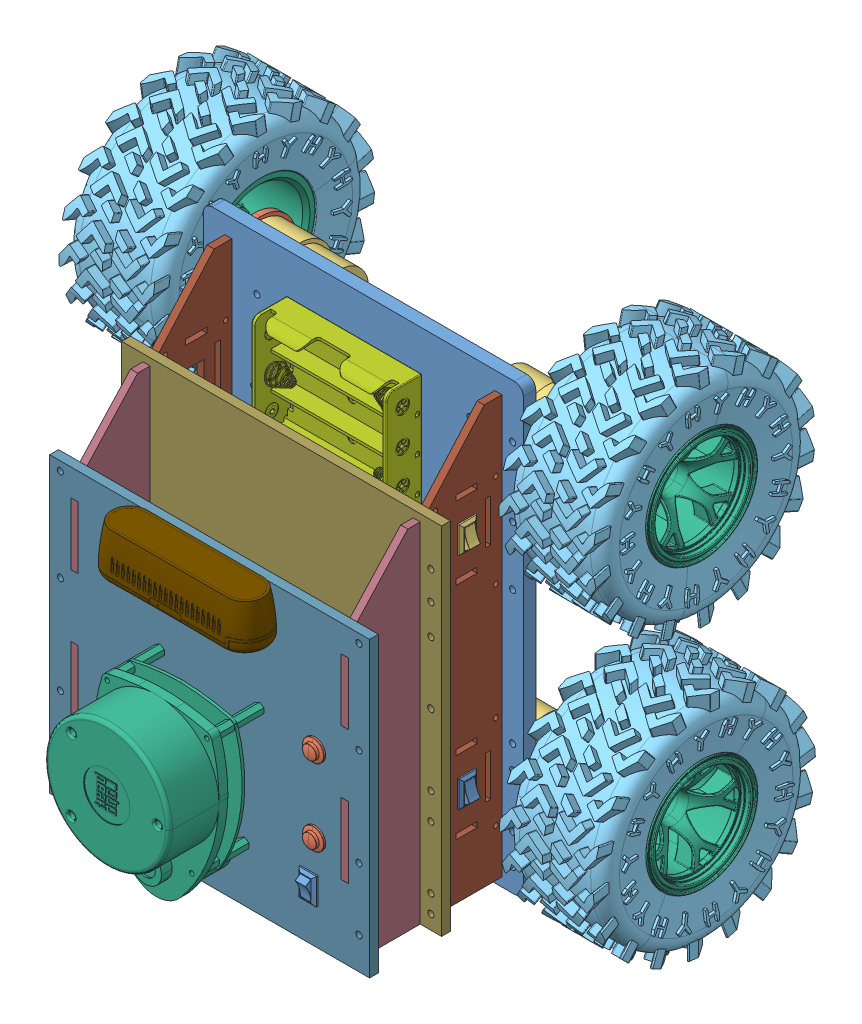
SolidWorks assembly Assem1, configuration Default. Lengths in mm. (continued)
Mates (geometry in assembly coordinates): (continued)
- Coincident108: coincident anti-aligned: plane of BTS_driver-4 through (-152.8182 1209.5505 -471.1522) normal (0 0 1); plane of Copy of hexagonal_spacer_FF_M3_H05_HEX5_pass_through.step^Assem1-4 through (-175.8052 1191.8975 -471.1522) normal (0 0 -1)
- Concentric77: concentric anti-aligned: cylinder of BTS_driver-4 through (-175.8052 1227.4575 -470.3622) axis (0 0 -1) radius 1.75; cylinder of Copy of hexagonal_spacer_FF_M3_H05_HEX5_pass_through.step^Assem1-5 through (-175.8052 1227.4575 -470.8751) axis (0 0 1) radius 1.5
- Coincident109: coincident anti-aligned: plane of BTS_driver-4 through (-152.8182 1209.5505 -471.1522) normal (0 0 1); plane of Copy of hexagonal_spacer_FF_M3_H05_HEX5_pass_through.step^Assem1-5 through (-175.8052 1227.4575 -471.1522) normal (0 0 -1)
- Concentric78: concentric anti-aligned: cylinder of BTS_driver-4 through (-130.0852 1227.4575 -470.3622) axis (0 0 -1) radius 1.75; cylinder of Copy of hexagonal_spacer_FF_M3_H05_HEX5_pass_through.step^Assem1-6 through (-130.0852 1227.4575 -470.8751) axis (0 0 1) radius 1.5
- Coincident110: coincident anti-aligned: plane of BTS_driver-4 through (-152.8182 1209.5505 -471.1522) normal (0 0 1); plane of Copy of hexagonal_spacer_FF_M3_H05_HEX5_pass_through.step^Assem1-6 through (-130.0852 1227.4575 -471.1522) normal (0 0 -1)
- Concentric79: concentric anti-aligned: cylinder of BTS_driver-4 through (-130.0852 1191.8975 -470.3622) axis (0 0 -1) radius 1.75; cylinder of Copy of hexagonal_spacer_FF_M3_H05_HEX5_pass_through.step^Assem1-7 through (-130.0852 1191.8975 -470.8751) axis (0 0 1) radius 1.5
- Coincident111: coincident anti-aligned: plane of BTS_driver-4 through (-152.8182 1209.5505 -471.1522) normal (0 0 1); plane of Copy of hexagonal_spacer_FF_M3_H05_HEX5_pass_through.step^Assem1-7 through (-130.0852 1191.8975 -471.1522) normal (0 0 -1)
- Concentric80: concentric anti-aligned: cylinder of BTS_driver-2 through (-253.5052 1290.2975 -470.3622) axis (0 0 -1) radius 1.75; cylinder of Copy of hexagonal_spacer_FF_M3_H05_HEX5_pass_through.step^Assem1-13 through (-253.5052 1290.2975 -470.8751) axis (0 0 1) radius 1.5
- Coincident112: coincident anti-aligned: plane of BTS_driver-2 through (-230.7722 1272.6445 -471.1522) normal (0 0 1); plane of Copy of hexagonal_spacer_FF_M3_H05_HEX5_pass_through.step^Assem1-13 through (-253.5052 1290.2975 -471.1522) normal (0 0 -1)
- Coincident113: coincident anti-aligned: plane of BTS_driver-2 through (-230.7722 1272.6445 -471.1522) normal (0 0 1); plane of Copy of hexagonal_spacer_FF_M3_H05_HEX5_pass_through.step^Assem1-12 through (-207.7852 1290.2975 -471.1522) normal (0 0 -1)
- Concentric81: concentric anti-aligned: cylinder of BTS_driver-2 through (-207.7852 1290.2975 -470.3622) axis (0 0 -1) radius 1.75; cylinder of Copy of hexagonal_spacer_FF_M3_H05_HEX5_pass_through.step^Assem1-12 through (-207.7852 1290.2975 -470.8751) axis (0 0 1) radius 1.5
- Concentric82: concentric anti-aligned: cylinder of BTS_driver-2 through (-207.7852 1254.7375 -470.3622) axis (0 0 -1) radius 1.75; cylinder of Copy of hexagonal_spacer_FF_M3_H05_HEX5_pass_through.step^Assem1-11 through (-207.7852 1254.7375 -470.8751) axis (0 0 1) radius 1.5
- Coincident114: coincident anti-aligned: plane of BTS_driver-2 through (-230.7722 1272.6445 -471.1522) normal (0 0 1); plane of Copy of hexagonal_spacer_FF_M3_H05_HEX5_pass_through.step^Assem1-11 through (-207.7852 1254.7375 -471.1522) normal (0 0 -1)
- Concentric83: concentric anti-aligned: cylinder of BTS_driver-2 through (-253.5052 1254.7375 -470.3622) axis (0 0 -1) radius 1.75; cylinder of Copy of hexagonal_spacer_FF_M3_H05_HEX5_pass_through.step^Assem1-10 through (-253.5052 1254.7375 -470.8751) axis (0 0 1) radius 1.5
- Coincident115: coincident anti-aligned: plane of BTS_driver-2 through (-230.7722 1272.6445 -471.1522) normal (0 0 1); plane of Copy of hexagonal_spacer_FF_M3_H05_HEX5_pass_through.step^Assem1-10 through (-253.5052 1254.7375 -471.1522) normal (0 0 -1)
- Concentric84: concentric anti-aligned: cylinder of BTS_driver-5 through (-207.7852 1227.4575 -470.3622) axis (0 0 -1) radius 1.75; cylinder of Copy of hexagonal_spacer_FF_M3_H05_HEX5_pass_through.step^Assem1-14 through (-207.7852 1227.4575 -470.8751) axis (0 0 1) radius 1.5
- Concentric86: concentric anti-aligned: cylinder of BTS_driver-5 through (-253.5052 1191.8975 -470.3622) axis (0 0 -1) radius 1.75; cylinder of Copy of hexagonal_spacer_FF_M3_H05_HEX5_pass_through.step^Assem1-15 through (-253.5052 1191.8975 -470.8751) axis (0 0 1) radius 1.5
- Concentric87: concentric aligned: cylinder of BTS_driver-5 through (-207.7852 1191.8975 -470.3622) axis (0 0 -1) radius 1.75; circle of Copy of hexagonal_spacer_FF_M3_H05_HEX5_pass_through.step^Assem1-9
- Coincident116: coincident anti-aligned: plane of BTS_driver-5 through (-230.7722 1209.8045 -471.1522) normal (0 0 1); plane of Copy of hexagonal_spacer_FF_M3_H05_HEX5_pass_through.step^Assem1-14 through (-207.7852 1227.4575 -471.1522) normal (0 0 -1)
- Coincident117: coincident anti-aligned: plane of BTS_driver-5 through (-230.7722 1209.8045 -471.1522) normal (0 0 1); plane of Copy of hexagonal_spacer_FF_M3_H05_HEX5_pass_through.step^Assem1-9 through (-207.7852 1191.8975 -471.1522) normal (0 0 -1)
- Coincident118: coincident anti-aligned: plane of BTS_driver-5 through (-230.7722 1209.8045 -471.1522) normal (0 0 1); plane of Copy of hexagonal_spacer_FF_M3_H05_HEX5_pass_through.step^Assem1-15 through (-253.5052 1191.8975 -471.1522) normal (0 0 -1)
- Coincident120: coincident anti-aligned: plane of Tam_lot_motorLon-2 through (-191.7952 1241.0975 -466.1522) normal (0 0 -1); plane of Copy of hexagonal_spacer_FF_M3_H05_HEX5_pass_through.step^Assem1-6 through (-130.0852 1227.4575 -466.1522) normal (0 0 1)
- Coincident121: coincident anti-aligned: plane of Tam_lot_motorLon-2 through (-191.7952 1241.0975 -466.1522) normal (0 0 -1); plane of Copy of hexagonal_spacer_FF_M3_H05_HEX5_pass_through.step^Assem1-2 through (-130.0852 1254.7375 -466.1522) normal (0 0 1)
- Coincident122: coincident anti-aligned: plane of Tam_lot_motorLon-2 through (-191.7952 1241.0975 -466.1522) normal (0 0 -1); plane of Copy of hexagonal_spacer_FF_M3_H05_HEX5_pass_through.step^Assem1-14 through (-207.7852 1227.4575 -466.1522) normal (0 0 1)
- Concentric88: concentric anti-aligned: cylinder of BTS_driver-5 through (-253.5052 1227.4575 -470.3622) axis (0 0 -1) radius 1.75; cylinder of Copy of hexagonal_spacer_FF_M3_H05_HEX5_pass_through.step^Assem1-16 through (-253.5052 1227.4575 -470.8751) axis (0 0 1) radius 1.5
- Coincident124: coincident anti-aligned: plane of BTS_driver-5 through (-230.7722 1209.8045 -471.1522) normal (0 0 1); plane of Copy of hexagonal_spacer_FF_M3_H05_HEX5_pass_through.step^Assem1-16 through (-253.5052 1227.4575 -471.1522) normal (0 0 -1)
- Coincident125: coincident anti-aligned: plane of Tam_lot_motorLon-2 through (-191.7952 1241.0975 -466.1522) normal (0 0 -1); plane of Copy of hexagonal_spacer_FF_M3_H05_HEX5_pass_through.step^Assem1-10 through (-253.5052 1254.7375 -466.1522) normal (0 0 1)
- Parallel37: parallel anti-aligned: line of BTS_driver-2 through (-256.2992 1252.1975 -472.7322) axis (1 0 0); line of BTS_driver-5 through (-205.2452 1230.2515 -472.7322) axis (-1 0 0)
- Parallel38: parallel anti-aligned: line of BTS_driver-2 through (-205.2452 1252.1975 -472.7322) axis (0 1 0); line of BTS_driver-3 through (-178.3452 1292.8375 -472.7322) axis (0 -1 0)
- Parallel39: parallel anti-aligned: line of BTS_driver-4 through (-178.3452 1229.9975 -472.7322) axis (0 -1 0); line of BTS_driver-5 through (-205.2452 1189.3575 -472.7322) axis (0 1 0)
- Parallel40: parallel aligned: line of Tam_lot_motorLon-2 through (-281.7952 1361.0975 -466.1522) axis (0 -1 0); line of BTS_driver-2 through (-256.2992 1293.0915 -472.7322) axis (0 -1 0)
- Concentric91: concentric anti-aligned: cylinder of Tam_lot_motorLon-2 through (-253.5052 1227.4575 -454.2591) axis (0 0 -1) radius 1.73; cylinder of Copy of hexagonal_spacer_FF_M3_H05_HEX5_pass_through.step^Assem1-16 through (-253.5052 1227.4575 -470.8751) axis (0 0 1) radius 1.5
- Concentric92: concentric anti-aligned: cylinder of Tam_lot_motorLon-2 through (-253.5052 1290.2975 -454.2591) axis (0 0 -1) radius 1.73; cylinder of Copy of hexagonal_spacer_FF_M3_H05_HEX5_pass_through.step^Assem1-13 through (-253.5052 1290.2975 -470.8751) axis (0 0 1) radius 1.5
- Concentric93: concentric anti-aligned: cylinder of Tam_lot_motorLon-2 through (-175.8052 1227.4575 -454.2591) axis (0 0 -1) radius 1.73; cylinder of Copy of hexagonal_spacer_FF_M3_H05_HEX5_pass_through.step^Assem1-5 through (-175.8052 1227.4575 -470.8751) axis (0 0 1) radius 1.5
- Concentric94: concentric anti-aligned: cylinder of Tam_lot_motorLon-2 through (-175.8052 1254.7375 -454.2591) axis (0 0 -1) radius 1.73; cylinder of Copy of hexagonal_spacer_FF_M3_H05_HEX5_pass_through.step^Assem1-1 through (-175.8052 1254.7375 -470.8751) axis (0 0 1) radius 1.5
- Concentric95: concentric anti-aligned: cylinder of LM2596-4 through (-151.9594 1232.9725 -452.4522) axis (0 0 -1) radius 1.475; cylinder of Copy of hexagonal_spacer_FF_M3_H05_HEX5_pass_through.step^Assem1-22 through (-151.9594 1232.9725 -458.8751) axis (0 0 1) radius 1.5
- Coincident133: coincident anti-aligned: plane of LM2596-4 through (-167.0594 1241.0975 -454.1522) normal (0 0 -1); plane of Copy of hexagonal_spacer_FF_M3_H05_HEX5_pass_through.step^Assem1-22 through (-151.9594 1232.9725 -454.1522) normal (0 0 1)
- Concentric96: concentric anti-aligned: cylinder of Copy of hexagonal_spacer_FF_M3_H05_HEX5_pass_through.step^Assem1-17 through (-182.1594 1249.2225 -458.8751) axis (0 0 1) radius 1.5; cylinder of LM2596-4 through (-182.1594 1249.2225 -452.4522) axis (0 0 -1) radius 1.475
- Coincident134: coincident anti-aligned: plane of Copy of hexagonal_spacer_FF_M3_H05_HEX5_pass_through.step^Assem1-17 through (-182.1594 1249.2225 -454.1522) normal (0 0 1); plane of LM2596-4 through (-167.0594 1241.0975 -454.1522) normal (0 0 -1)
- Concentric98: concentric anti-aligned: cylinder of Copy of hexagonal_spacer_FF_M3_H05_HEX5_pass_through.step^Assem1-18 through (-202.0152 1232.9725 -458.8751) axis (0 0 1) radius 1.5; cylinder of LM2596-3 through (-202.0152 1232.9725 -452.4522) axis (0 0 -1) radius 1.475
- Coincident135: coincident anti-aligned: plane of Copy of hexagonal_spacer_FF_M3_H05_HEX5_pass_through.step^Assem1-18 through (-202.0152 1232.9725 -454.1522) normal (0 0 1); plane of LM2596-3 through (-217.1152 1241.0975 -454.1522) normal (0 0 -1)
- Coincident136: coincident anti-aligned: plane of Copy of hexagonal_spacer_FF_M3_H05_HEX5_pass_through.step^Assem1-21 through (-232.2152 1249.2225 -454.1522) normal (0 0 1); plane of LM2596-3 through (-217.1152 1241.0975 -454.1522) normal (0 0 -1)
- Concentric99: concentric anti-aligned: cylinder of Copy of hexagonal_spacer_FF_M3_H05_HEX5_pass_through.step^Assem1-21 through (-232.2152 1249.2225 -458.8751) axis (0 0 1) radius 1.5; cylinder of LM2596-3 through (-232.2152 1249.2225 -452.4522) axis (0 0 -1) radius 1.475
- Coincident137: coincident anti-aligned: plane of Tam_lot_motorLon-2 through (-191.7952 1241.0975 -459.1522) normal (0 0 1); plane of Copy of hexagonal_spacer_FF_M3_H05_HEX5_pass_through.step^Assem1-21 through (-232.2152 1249.2225 -459.1522) normal (0 0 -1)
- Coincident138: coincident anti-aligned: plane of Tam_lot_motorLon-2 through (-191.7952 1241.0975 -459.1522) normal (0 0 1); plane of Copy of hexagonal_spacer_FF_M3_H05_HEX5_pass_through.step^Assem1-22 through (-151.9594 1232.9725 -459.1522) normal (0 0 -1)
- Parallel41: parallel aligned: plane of Tam_lot_motorLon-2 through (-281.7952 1116.0975 -459.1522) normal (0 -1 0); plane of Copy of 18650 Cell Holder^Assem1-1 through (-231.0952 1140.7125 -454.1522) normal (0 -1 0)
- Parallel42: parallel aligned: plane of Tam_lot_motorLon-2 through (-281.7952 1116.0975 -459.1522) normal (0 -1 0); plane of Copy of 18650 Cell Holder^Assem1-1 through (-231.0952 1140.7125 -454.1522) normal (0 -1 0)
- Parallel43: parallel aligned: plane of Tam_lot_motorLon-2 through (-281.7952 1366.0975 -459.1522) normal (0 1 0); plane of khay_pin-4/Assem_done(2)^khay_pin-1/18650 Cell Holder^Assem_done(2)_khay_pin-1 through (-152.4952 1341.4825 -459.1522) normal (0 1 0)
- Concentric106: concentric aligned: cylinder of Tam_lot_motorLon-2 through (-202.0152 1232.9725 -454.2591) axis (0 0 -1) radius 1.73; cylinder of LM2596-3 through (-202.0152 1232.9725 -452.4522) axis (0 0 -1) radius 1.475
- Concentric107: concentric aligned: cylinder of Tam_lot_motorLon-2 through (-232.2152 1249.2225 -454.2591) axis (0 0 -1) radius 1.73; cylinder of LM2596-3 through (-232.2152 1249.2225 -452.4522) axis (0 0 -1) radius 1.475
- Concentric108: concentric anti-aligned: cylinder of Tam_lot_motorLon-2 through (-182.1594 1249.2225 -454.2591) axis (0 0 -1) radius 1.73; cylinder of Copy of hexagonal_spacer_FF_M3_H05_HEX5_pass_through.step^Assem1-17 through (-182.1594 1249.2225 -456.6522) axis (0 0 1) radius 1.5
- Concentric109: concentric anti-aligned: cylinder of Tam_lot_motorLon-2 through (-151.9594 1232.9725 -454.2591) axis (0 0 -1) radius 1.73; cylinder of Copy of hexagonal_spacer_FF_M3_H05_HEX5_pass_through.step^Assem1-22 through (-151.9594 1232.9725 -458.8751) axis (0 0 1) radius 1.5
- Parallel45: parallel aligned: plane of Tam_lot_motorLon-2 through (-281.7952 1366.0975 -459.1522) normal (0 1 0); plane of khay_pin-4/Assem_done(2)^khay_pin-1/18650 Cell Holder^Assem_done(2)_khay_pin-1 through (-152.4952 1341.4825 -459.1522) normal (0 1 0)
- Parallel46: parallel aligned: plane of Tam_lot_motorLon-2 through (-101.7952 1366.0975 -459.1522) normal (1 0 0); plane of mat_ben_co_sac-2 through (-113.7952 1238.5975 -459.1522) normal (1 0 0)
- Coincident155: coincident anti-aligned: plane of Tam_lot_motorLon-2 through (-113.7952 1121.0975 -478.8013) normal (0 1 0); plane of mat_ben_co_sac-2 through (-113.7952 1121.0975 -459.1522) normal (0 -1 0)
- Coincident156: coincident anti-aligned: plane of Tam_lot_motorLon-2 through (-113.7952 1133.0975 -478.8013) normal (-1 0 0); plane of mat_ben_co_sac-2 through (-113.7952 1238.5975 -459.1522) normal (1 0 0)
- Coincident157: coincident aligned: plane of Tam_lot_motorLon-2 through (-191.7952 1241.0975 -466.1522) normal (0 0 -1); plane of mat_ben_co_sac-2 through (-113.7952 1133.0975 -466.1522) normal (0 0 -1)
- Coincident158: coincident aligned: plane of Tam_lot_motorLon-2 through (-191.7952 1241.0975 -466.1522) normal (0 0 -1); plane of mat_ben_co_sac-1 through (-265.7952 1133.0975 -466.1522) normal (0 0 -1)
- Parallel47: parallel aligned: plane of Tam_lot_motorLon-2 through (-281.7952 1116.0975 -459.1522) normal (0 -1 0); plane of mat_ben_co_sac-1 through (-265.7952 1121.0975 -459.1522) normal (0 -1 0)
- Coincident160: coincident anti-aligned: plane of Tam_lot_motorLon-2 through (-269.7952 1133.0975 -478.8013) normal (1 0 0); plane of mat_ben_co_sac-1 through (-269.7952 1238.5975 -459.1522) normal (-1 0 0)
- Coincident161: coincident anti-aligned: plane of Tam_lot_motorLon-2 through (-269.7952 1121.0975 -478.8013) normal (0 1 0); plane of mat_ben_co_sac-1 through (-265.7952 1121.0975 -459.1522) normal (0 -1 0)
- Coincident162: coincident anti-aligned: plane of mat_ben_co_sac-1 through (-269.7952 1238.5975 -459.1522) normal (-1 0 0); plane of tang2_2-2 through (-269.7952 1216.0975 -438.5483) normal (1 0 0)
- Coincident163: coincident anti-aligned: plane of mat_ben_co_sac-1 through (-265.7952 1301.0975 -413.1522) normal (0 1 0); plane of tang2_2-2 through (-265.7952 1301.0975 -433.6764) normal (0 -1 0)
- Coincident164: coincident aligned: plane of mat_ben_co_sac-2 through (-113.7952 1146.0975 -413.1522) normal (0 0 1); plane of tang2_2-2 through (-191.7952 1221.0975 -413.1522) normal (0 0 1)
- Coincident166: coincident anti-aligned: plane of tang2_2-2 through (-265.7952 1317.0975 -428.9226) normal (0 -1 0); plane of mat_ben_tang_2-1 through (-265.7952 1317.0975 -413.1522) normal (0 1 0)
- Coincident167: coincident anti-aligned: plane of tang2_2-2 through (-269.7952 1317.0975 -428.9226) normal (1 0 0); plane of mat_ben_tang_2-1 through (-269.7952 1221.0975 -413.1522) normal (-1 0 0)
- Coincident170: coincident aligned: plane of tang2_2-2 through (-191.7952 1221.0975 -418.1522) normal (0 0 -1); plane of mat_ben_tang_2-1 through (-265.7952 1311.0975 -418.1522) normal (0 0 -1)
- Coincident171: coincident anti-aligned: plane of tang2_2-2 through (-117.7952 1317.0975 -428.9226) normal (0 -1 0); plane of mat_ben_tang_2-2 through (-113.7952 1317.0975 -413.1522) normal (0 1 0)
- Coincident172: coincident anti-aligned: plane of tang2_2-2 through (-117.7952 1311.0975 -428.9226) normal (1 0 0); plane of mat_ben_tang_2-2 through (-117.7952 1221.0975 -413.1522) normal (-1 0 0)
- Coincident173: coincident aligned: plane of tang2_2-2 through (-191.7952 1221.0975 -418.1522) normal (0 0 -1); plane of mat_ben_tang_2-2 through (-113.7952 1125.0975 -418.1522) normal (0 0 -1)
- Coincident174: coincident anti-aligned: plane of mat_ben_tang_2-2 through (-113.7952 1271.0975 -372.6522) normal (0 1 0); plane of tang_3-1 through (-117.7952 1271.0975 -412.8801) normal (0 -1 0)
- Coincident175: coincident anti-aligned: plane of mat_ben_tang_2-2 through (-113.7952 1221.0975 -413.1522) normal (1 0 0); plane of tang_3-1 through (-113.7952 1161.0975 -417.8517) normal (-1 0 0)
- Coincident177: coincident aligned: plane of mat_ben_tang_2-2 through (-113.7952 1161.0975 -372.6522) normal (0 0 1); plane of tang_3-1 through (-191.7952 1203.5975 -372.6522) normal (0 0 1)
- Concentric121: concentric anti-aligned: cylinder of tang2_2-2 through (-167.2952 1217.5975 -422.3949) axis (0 0 1) radius 1.5; cylinder of Copy (4) of hexagonal_spacer_FF_M3_H05_HEX5_pass_through.step^Assem1-4 through (-167.2952 1217.5975 -408.4294) axis (0 0 -1) radius 1.5
- Concentric122: concentric anti-aligned: cylinder of tang2_2-2 through (-216.2952 1217.5975 -422.3949) axis (0 0 1) radius 1.5; cylinder of Copy (2) of hexagonal_spacer_FF_M3_H05_HEX5_pass_through.step^Assem1-2 through (-216.2952 1217.5975 -408.4294) axis (0 0 -1) radius 1.5
- Coincident182: coincident anti-aligned: plane of tang2_2-2 through (-191.7952 1221.0975 -413.1522) normal (0 0 1); plane of Copy (4) of hexagonal_spacer_FF_M3_H05_HEX5_pass_through.step^Assem1-4 through (-167.2952 1217.5975 -413.1522) normal (0 0 -1)
- Coincident187: coincident anti-aligned: plane of tang_3-1 through (-191.7952 1203.5975 -372.6522) normal (0 0 1); plane of IntelRealsense_D435_Multibody-1 through (-162.0261 1272.6733 -372.6522) normal (0 0 -1)
- Coincident188: coincident anti-aligned: plane of mat_ben_co_sac-2 through (-134.2257 1167.0975 -434.8522) normal (0 0 -1); plane of swith_on_off-1/Assem_done(2)^swith_on_off-1/Switch on off^Assem_done(2)_swith_on_off-1 through (-111.7952 1180.9706 -434.8522) normal (0 0 1)
- Coincident190: coincident anti-aligned: plane of mat_ben_co_sac-2 through (-113.7952 1238.5975 -459.1522) normal (1 0 0); plane of swith_on_off-1/Assem_done(2)^swith_on_off-1/Switch on off^Assem_done(2)_swith_on_off-1 through (-113.7952 1167.3306 -434.8522) normal (-1 0 0)
- Lock3: lock: unknown of mat_ben_co_sac-2; unknown of swith_on_off-1/Assem_done(2)^swith_on_off-1/Switch on off^Assem_done(2)_swith_on_off-1
- Coincident192: coincident anti-aligned: plane of mat_ben_co_sac-2 through (-134.2257 1291.0975 -434.8522) normal (0 0 -1); plane of Copy of Switch on off^Assem1-1 through (-111.7952 1304.8258 -434.8522) normal (0 0 1)
- Coincident193: coincident anti-aligned: plane of mat_ben_co_sac-2 through (-113.7952 1238.5975 -459.1522) normal (1 0 0); plane of Copy of Switch on off^Assem1-1 through (-113.7952 1291.1858 -434.8522) normal (-1 0 0)
- Lock4: lock: unknown of mat_ben_co_sac-2; unknown of Copy of Switch on off^Assem1-1
- Concentric123: concentric anti-aligned: cylinder of hexagone M3-2/Assem_done(2)^hexagone M3-1/hexagonal_spacer_FF_M3_H05_HEX5_pass_through.step^Assem_done(2)_hexagone M3-3 through (-167.2952 1159.5975 -409.4294) axis (0 0 -1) radius 1.5; cylinder of raspberry pi 4-2/Assem_done(2)^raspberry pi 4-1/Raspberry Pi 4 Model B^Assem_done(2)_raspberry pi 4-1 through (-167.2952 1159.5975 -406.5622) axis (0 0 1) radius 1.35
- Concentric124: concentric anti-aligned: cylinder of Copy (3) of hexagonal_spacer_FF_M3_H05_HEX5_pass_through.step^Assem1-3 through (-216.2952 1159.5975 -409.2374) axis (0 0 -1) radius 1.5; cylinder of raspberry pi 4-2/Assem_done(2)^raspberry pi 4-1/Raspberry Pi 4 Model B^Assem_done(2)_raspberry pi 4-1 through (-216.2952 1159.5975 -406.5622) axis (0 0 1) radius 1.35
- Concentric125: concentric anti-aligned: cylinder of Copy (2) of hexagonal_spacer_FF_M3_H05_HEX5_pass_through.step^Assem1-2 through (-216.2952 1217.5975 -408.4294) axis (0 0 -1) radius 1.5; cylinder of raspberry pi 4-2/Assem_done(2)^raspberry pi 4-1/Raspberry Pi 4 Model B^Assem_done(2)_raspberry pi 4-1 through (-216.2952 1217.5975 -406.5622) axis (0 0 1) radius 1.35
- Concentric126: concentric anti-aligned: cylinder of tang2_2-2 through (-216.2952 1159.5975 -422.3949) axis (0 0 1) radius 1.5; cylinder of Copy (3) of hexagonal_spacer_FF_M3_H05_HEX5_pass_through.step^Assem1-3 through (-216.2952 1159.5975 -409.2374) axis (0 0 -1) radius 1.5
- Concentric127: concentric anti-aligned: cylinder of tang2_2-2 through (-216.2952 1217.5975 -422.3949) axis (0 0 1) radius 1.5; cylinder of Copy (2) of hexagonal_spacer_FF_M3_H05_HEX5_pass_through.step^Assem1-2 through (-216.2952 1217.5975 -408.4294) axis (0 0 -1) radius 1.5
- Coincident194: coincident anti-aligned: plane of tang2_2-2 through (-191.7952 1221.0975 -413.1522) normal (0 0 1); plane of Copy (2) of hexagonal_spacer_FF_M3_H05_HEX5_pass_through.step^Assem1-2 through (-216.2952 1217.5975 -413.1522) normal (0 0 -1)
- Coincident195: coincident anti-aligned: plane of Copy (2) of hexagonal_spacer_FF_M3_H05_HEX5_pass_through.step^Assem1-2 through (-216.2952 1217.5975 -408.1522) normal (0 0 1); plane of raspberry pi 4-2/Assem_done(2)^raspberry pi 4-1/Raspberry Pi 4 Model B^Assem_done(2)_raspberry pi 4-1 through (-216.2952 1217.5975 -408.1522) normal (0 0 -1)
- Concentric128: concentric aligned: cylinder of LM2596-5 through (-149.9202 1143.4975 -406.4522) axis (0 0 -1) radius 1.475; cylinder of Copy (5) of hexagonal_spacer_FF_M3_H05_HEX5_pass_through.step^Assem1-2 through (-149.9202 1143.4975 -410.6522) axis (0 0 -1) radius 1.5
- Concentric129: concentric anti-aligned: cylinder of LM2596-5 through (-133.6702 1173.6975 -406.4522) axis (0 0 -1) radius 1.475; circle of Copy (5) of hexagonal_spacer_FF_M3_H05_HEX5_pass_through.step^Assem1-1
- Coincident196: coincident anti-aligned: plane of LM2596-5 through (-141.7952 1158.5975 -408.1522) normal (0 0 -1); plane of Copy (5) of hexagonal_spacer_FF_M3_H05_HEX5_pass_through.step^Assem1-2 through (-149.9202 1143.4975 -408.1522) normal (0 0 1)
- Coincident197: coincident anti-aligned: plane of LM2596-5 through (-141.7952 1158.5975 -408.1522) normal (0 0 -1); plane of Copy (5) of hexagonal_spacer_FF_M3_H05_HEX5_pass_through.step^Assem1-1 through (-133.6702 1173.6975 -408.1522) normal (0 0 1)
- Concentric130: concentric anti-aligned: cylinder of tang2_2-2 through (-133.6702 1173.6975 -423.0454) axis (0 0 1) radius 1.73; cylinder of Copy (5) of hexagonal_spacer_FF_M3_H05_HEX5_pass_through.step^Assem1-1 through (-133.6702 1173.6975 -408.4294) axis (0 0 -1) radius 1.5
- Concentric131: concentric anti-aligned: cylinder of tang2_2-2 through (-149.9202 1143.4975 -423.0454) axis (0 0 1) radius 1.73; cylinder of Copy (5) of hexagonal_spacer_FF_M3_H05_HEX5_pass_through.step^Assem1-2 through (-149.9202 1143.4975 -408.4294) axis (0 0 -1) radius 1.5
- Coincident198: coincident anti-aligned: plane of tang2_2-2 through (-191.7952 1221.0975 -413.1522) normal (0 0 1); plane of Copy (5) of hexagonal_spacer_FF_M3_H05_HEX5_pass_through.step^Assem1-2 through (-149.9202 1143.4975 -413.1522) normal (0 0 -1)
- Coincident199: coincident anti-aligned: plane of tang_3-1 through (-191.7952 1203.5975 -372.6522) normal (0 0 1); plane of lidarA1-2/Assem_done(2)^lidarA1-1/rplidar_main_По умолчанию^Assem_done(2)_lidarA1-1 through (-192.0863 1179.5544 -372.6522) normal (0 0 -1)
- Lock5: lock: unknown of tang_3-1; unknown of lidarA1-2/Assem_done(2)^lidarA1-1/rplidar_main_По умолчанию^Assem_done(2)_lidarA1-1
- Concentric136: concentric aligned: cylinder of tang_3-1 through (-132.5348 1174.1165 -356.2218) axis (0 0 -1) radius 5.25; cylinder of swith_hold-2/Assem_done(2)^swith_hold-1/Push_main_Défaut^Assem_done(2)_swith_hold-1 through (-132.5348 1174.1165 -387.6522) axis (0 0 -1) radius 4.84
- Coincident201: coincident anti-aligned: plane of tang_3-1 through (-191.7952 1203.5975 -372.6522) normal (0 0 1); plane of swith_hold-2/Assem_done(2)^swith_hold-1/Push_main_Défaut^Assem_done(2)_swith_hold-1 through (-132.5348 1174.1165 -372.6522) normal (0 0 -1)
- Concentric137: concentric aligned: cylinder of tang_3-1 through (-132.5348 1217.2194 -356.2218) axis (0 0 -1) radius 5.25; cylinder of swith_hold-3/Assem_done(2)^swith_hold-1/Push_main_Défaut^Assem_done(2)_swith_hold-1 through (-132.5348 1217.2194 -387.6522) axis (0 0 -1) radius 4.84
- Coincident202: coincident anti-aligned: plane of tang_3-1 through (-191.7952 1203.5975 -372.6522) normal (0 0 1); plane of swith_hold-3/Assem_done(2)^swith_hold-1/Push_main_Défaut^Assem_done(2)_swith_hold-1 through (-132.5348 1217.2194 -372.6522) normal (0 0 -1)
- Coincident203: coincident anti-aligned: plane of tang_3-1 through (-140.0952 1155.4801 -356.2218) normal (1 0 0); plane of swith_on_off-2/Assem_done(2)^swith_on_off-1/Switch on off^Assem_done(2)_swith_on_off-1 through (-140.0952 1142.1429 -370.6522) normal (-1 0 0)
- Coincident204: coincident anti-aligned: plane of tang_3-1 through (-191.7952 1203.5975 -372.6522) normal (0 0 1); plane of swith_on_off-2/Assem_done(2)^swith_on_off-1/Switch on off^Assem_done(2)_swith_on_off-1 through (-131.5652 1155.7829 -372.6522) normal (0 0 -1)
- Lock6: lock: unknown of tang_3-1; unknown of swith_on_off-2/Assem_done(2)^swith_on_off-1/Switch on off^Assem_done(2)_swith_on_off-1
- Coincident206: coincident anti-aligned: plane of tang_3-1 through (-191.7952 1203.5975 -372.6522) normal (0 0 1); plane of IntelRealsense_D435_Multibody-1 through (-162.0261 1272.6733 -372.6522) normal (0 0 -1)
- Concentric138: concentric aligned: cylinder of tang_3-1 through (-191.7952 1274.0975 -367.7591) axis (0 0 -1) radius 1.73; cylinder of IntelRealsense_D435_Multibody-1 through (-191.7952 1274.0975 -372.6522) axis (0 0 -1) radius 2.5527
- Concentric139: concentric aligned: cylinder of Copy of hexagonal_spacer_FF_M3_H05_HEX5_pass_through.step^Assem1-36 through (-191.7952 1143.9375 -456.6522) axis (0 0 1) radius 1.5; cylinder of 18650 Battery Holder 4x-3 through (-191.7952 1143.9375 -454.1532) axis (0 0 1) radius 1.45
- Coincident207: coincident anti-aligned: plane of Copy of hexagonal_spacer_FF_M3_H05_HEX5_pass_through.step^Assem1-36 through (-191.7952 1143.9375 -454.1522) normal (0 0 1); plane of 18650 Battery Holder 4x-3 through (-153.7952 1133.4375 -454.1522) normal (0 0 -1)
- Concentric140: concentric aligned: cylinder of Copy of hexagonal_spacer_FF_M3_H05_HEX5_pass_through.step^Assem1-33 through (-191.7952 1202.4375 -458.8751) axis (0 0 1) radius 1.5; cylinder of 18650 Battery Holder 4x-3 through (-191.7952 1202.4375 -454.1532) axis (0 0 1) radius 1.45
- Coincident208: coincident anti-aligned: plane of Copy of hexagonal_spacer_FF_M3_H05_HEX5_pass_through.step^Assem1-33 through (-191.7952 1202.4375 -454.1522) normal (0 0 1); plane of 18650 Battery Holder 4x-3 through (-153.7952 1133.4375 -454.1522) normal (0 0 -1)
- Concentric141: concentric aligned: cylinder of Copy of hexagonal_spacer_FF_M3_H05_HEX5_pass_through.step^Assem1-34 through (-191.7952 1279.7575 -458.8751) axis (0 0 1) radius 1.5; cylinder of 18650 Battery Holder 4x-2 through (-191.7952 1279.7575 -454.1532) axis (0 0 1) radius 1.45
- Coincident209: coincident aligned: circle of Copy of hexagonal_spacer_FF_M3_H05_HEX5_pass_through.step^Assem1-34; plane of 18650 Battery Holder 4x-2 through (-153.7952 1269.2575 -454.1522) normal (0 0 -1)
- Concentric142: concentric aligned: cylinder of Copy of hexagonal_spacer_FF_M3_H05_HEX5_pass_through.step^Assem1-35 through (-191.7952 1338.2575 -458.8751) axis (0 0 1) radius 1.5; cylinder of 18650 Battery Holder 4x-2 through (-191.7952 1338.2575 -454.1532) axis (0 0 1) radius 1.45
- Coincident210: coincident anti-aligned: plane of Copy of hexagonal_spacer_FF_M3_H05_HEX5_pass_through.step^Assem1-35 through (-191.7952 1338.2575 -454.1522) normal (0 0 1); plane of 18650 Battery Holder 4x-2 through (-153.7952 1269.2575 -454.1522) normal (0 0 -1)
- Concentric143: concentric anti-aligned: cylinder of Tam_lot_motorLon-2 through (-191.7952 1279.7575 -454.2591) axis (0 0 -1) radius 1.73; cylinder of Copy of hexagonal_spacer_FF_M3_H05_HEX5_pass_through.step^Assem1-34 through (-191.7952 1279.7575 -458.8751) axis (0 0 1) radius 1.5
- Concentric144: concentric anti-aligned: cylinder of Tam_lot_motorLon-2 through (-191.7952 1338.2575 -454.2591) axis (0 0 -1) radius 1.73; cylinder of Copy of hexagonal_spacer_FF_M3_H05_HEX5_pass_through.step^Assem1-35 through (-191.7952 1338.2575 -458.8751) axis (0 0 1) radius 1.5
- Coincident211: coincident anti-aligned: plane of Tam_lot_motorLon-2 through (-191.7952 1241.0975 -459.1522) normal (0 0 1); plane of Copy of hexagonal_spacer_FF_M3_H05_HEX5_pass_through.step^Assem1-35 through (-191.7952 1338.2575 -459.1522) normal (0 0 -1)
- Concentric145: concentric anti-aligned: cylinder of Tam_lot_motorLon-2 through (-191.7952 1202.4375 -454.2591) axis (0 0 -1) radius 1.73; cylinder of Copy of hexagonal_spacer_FF_M3_H05_HEX5_pass_through.step^Assem1-33 through (-191.7952 1202.4375 -458.8751) axis (0 0 1) radius 1.5
- Concentric146: concentric anti-aligned: cylinder of Tam_lot_motorLon-2 through (-191.7952 1143.9375 -454.2591) axis (0 0 -1) radius 1.73; cylinder of Copy of hexagonal_spacer_FF_M3_H05_HEX5_pass_through.step^Assem1-36 through (-191.7952 1143.9375 -458.8751) axis (0 0 1) radius 1.5
- Coincident212: coincident anti-aligned: plane of Tam_lot_motorLon-2 through (-191.7952 1241.0975 -459.1522) normal (0 0 1); plane of Copy of hexagonal_spacer_FF_M3_H05_HEX5_pass_through.step^Assem1-36 through (-191.7952 1143.9375 -459.1522) normal (0 0 -1)
